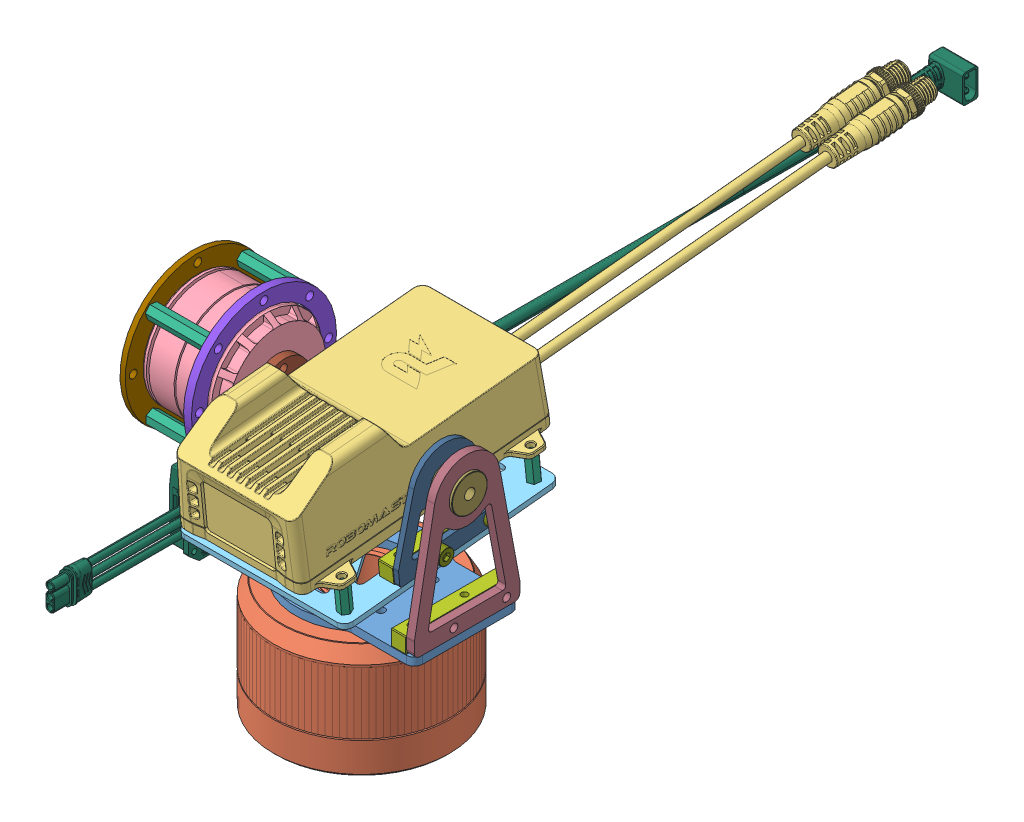
SolidWorks assembly 图传云台模块, configuration 默认. Lengths in mm.
Overall size (117.49 133.37 343.45).
28 component instances, 16 part files, 65 mates.
Components (placement in the parent):
- 6020电机传动板-1: 6020电机传动板 [默认] x (1 0 0) z (0 -1 0) size (80 50 3)
- RoboMaster GM6020 直流无刷电机-1: RoboMaster GM6020 直流无刷电机 [默认] at (0 72.0479 0) x (0.664685 0 -0.747124) z (0 1 0) size (66.7 66.7 45)
- RoboMaster 图传模块 VT02 2019-1: RoboMaster 图传模块 VT02 2019 [默认] at (0 34.0545 -1.0941) x (-1 0 0) z (0 0.099465 -0.995041) size (60 36.29 258.03)
- RoboMaster M3508直流无刷电机转子-1: RoboMaster M3508直流无刷电机转子 [默认] at (-11.659 32.3995 -13.3475) x (0 -0.790596 0.612338) z (-1 0 0) size (42 42 43.4)
- 图传安装板-1: 图传安装板 [默认] at (0 20.124 -2.4866) x (1 0 0) z (0 -0.995041 -0.099465) size (64 82 2)
- 304不锈钢柱-1: 304不锈钢柱 [M2*10] at (27 21.5184 33.8322) x (-0.601616 -0.079451 0.794824) z (0 -0.995041 -0.099465) size (4.62 4 10)
- 304不锈钢柱-2: 304不锈钢柱 [M2*10] at (-27 21.5184 33.8322) x (-0.601616 -0.079451 0.794824) z (0 -0.995041 -0.099465) size (4.62 4 10)
- 304不锈钢柱-3: 304不锈钢柱 [M2*10] at (27 28.6799 -37.8108) x (-0.956324 -0.029074 0.290859) z (0 -0.995041 -0.099465) size (4.62 4 10)
- 304不锈钢柱-4: 304不锈钢柱 [M2*10] at (-27 28.6799 -37.8108) x (0.570383 -0.081698 0.817306) z (0 -0.995041 -0.099465) size (4.62 4 10)
- 四孔直角转接件-1: 四孔直角转接件 [上交角件] at (-26 23.1091 -2.1882) x (1 0 0) z (0 -0.099465 0.995041) size (6 6 40)
- 四孔直角转接件-2: 四孔直角转接件 [上交角件] at (27 23.1091 -2.1882) x (1 0 0) z (0 -0.099465 0.995041) size (6 6 40)
- 云台转接板-1: 云台转接板 [默认] at (-37 45 0) x (0 0 1) z (-1 0 0) size (55 72.5 3.26)
- 3508定子安装板-1: 3508定子安装板 [默认] at (-64.1 45 0) x (0 0.707107 -0.707107) z (1 0 0) size (55 55 2)
- 云台旋转板-1: 云台旋转板 [默认] at (32 45 0) x (0 -0.099465 0.995041) z (-1 0 0) size (40 37.5 2)
- 3508传动板-1: 3508传动板 [默认] at (-32 45 0) x (0 0.099465 -0.995041) z (1 0 0) size (40 34.5 3)
- 法兰轴承-1: 法兰轴承 [4*12*4-1] at (41 45 0) x (0 0.036514 0.999333) z (0 -0.999333 0.036514) size (13.5 4 13.5)
- 转接板2-1: 转接板2 [默认] at (37 45 0) x (0 0 -1) z (1 0 0) size (40 57.5 3)
- 推力球轴承-1: 推力球轴承 [F4-9M 4*9*4] at (37 45 0) x (0 0.757396 -0.652956) z (0 0.652956 0.757396) size (9 4 9)
- 法兰轴承-2: 法兰轴承 [4*12*4-1] at (29 45 0) x (0 -0.234612 -0.972089) z (0 -0.972089 0.234612) size (13.5 4 13.5)
- 304不锈钢柱-5: 304不锈钢柱 [M3*22] at (-51 27.6759 17.3241) x (0 -0.514688 -0.857378) z (1 0 0) size (5.43 4.7 22)
- 304不锈钢柱-6: 304不锈钢柱 [M3*22] at (-51 27.6759 -17.3241) x (0 -0.372237 -0.928138) z (1 0 0) size (5.43 4.7 22)
- 304不锈钢柱-7: 304不锈钢柱 [M3*22] at (-51 62.3241 -17.3241) x (0 -0.251026 -0.96798) z (1 0 0) size (5.43 4.7 22)
- 304不锈钢柱-8: 304不锈钢柱 [M3*22] at (-51 62.3241 17.3241) x (0 -0.159705 -0.987165) z (1 0 0) size (5.43 4.7 22)
- 四孔直角转接件-3: 四孔直角转接件 [上交角件] at (34 3 0) size (6 6 40)
- 四孔直角转接件-4: 四孔直角转接件 [上交角件] at (-34 3 0) size (6 6 40)
- C620无刷电机调速器-1: C620无刷电机调速器 [默认] at (-45.4 6.2704 2.5313) x (0 0 1) z (0 1 0) size (343.45 13.81 26.13)
- 12.9级圆柱头螺钉-1: 12.9级圆柱头螺钉 [M3*8] at (35 22.6118 2.787) x (0 -0.455873 -0.890045) z (1 0 0) size (5.68 5.68 11)
- 12.9级圆柱头螺钉-2: 12.9级圆柱头螺钉 [M3*8] at (35 24.6011 -17.1138) x (0 -0.455873 -0.890045) z (1 0 0) size (5.68 5.68 11)
Mates (geometry in assembly coordinates):
- 重合1: coincident anti-aligned: plane of 6020电机传动板-1 through (0 -3 0) normal (0 -1 0); plane of RoboMaster GM6020 直流无刷电机-1 through (0 -3 0) normal (0 1 0)
- 同心1: concentric anti-aligned: cylinder of 6020电机传动板-1 through (0 -3 0) axis (0 1 0) radius 15; cylinder of RoboMaster GM6020 直流无刷电机-1 through (0 -0.95 0) axis (0 -1 0) radius 9
- 对称1: symmetric aligned: plane of RoboMaster 图传模块 VT02 2019-1 through (24 38.8289 -48.8561) normal (1 0 0); plane of RoboMaster 图传模块 VT02 2019-1 through (-24 29.2802 46.6679) normal (-1 0 0)
- 距离1: distance = 10 mm anti-aligned: plane of 图传安装板-1 through (0 20.124 -2.4866) normal (0 0.995041 0.099465); plane of RoboMaster 图传模块 VT02 2019-1 through (0 30.0744 -1.492) normal (0 -0.995041 -0.099465)
- 同心3: concentric aligned: cylinder of RoboMaster 图传模块 VT02 2019-1 through (27 26.4936 34.3295) axis (0 0.995041 0.099465) radius 1.35; cylinder of 图传安装板-1 through (27 14.5532 33.1359) axis (0 0.995041 0.099465) radius 1.25
- 同心4: concentric anti-aligned: cylinder of RoboMaster 图传模块 VT02 2019-1 through (-27 26.4936 34.3295) axis (0 -0.995041 -0.099465) radius 1.35; cylinder of 图传安装板-1 through (-27 14.5532 33.1359) axis (0 0.995041 0.099465) radius 1.25
- 重合3: coincident anti-aligned: plane of 图传安装板-1 through (0 20.124 -2.4866) normal (0 0.995041 0.099465); plane of 304不锈钢柱-1 through (27 16.5432 33.3349) normal (0 -0.995041 -0.099465)
- 同心5: concentric anti-aligned: cylinder of 图传安装板-1 through (27 14.5532 33.1359) axis (0 0.995041 0.099465) radius 1.25; cylinder of 304不锈钢柱-1 through (27 16.5432 33.3349) axis (0 -0.995041 -0.099465) radius 0.8
- 重合4: coincident anti-aligned: plane of 图传安装板-1 through (0 20.124 -2.4866) normal (0 0.995041 0.099465); plane of 304不锈钢柱-2 through (-27 16.5432 33.3349) normal (0 -0.995041 -0.099465)
- 同心6: concentric anti-aligned: cylinder of 图传安装板-1 through (-27 14.5532 33.1359) axis (0 0.995041 0.099465) radius 1.25; cylinder of 304不锈钢柱-2 through (-27 16.5432 33.3349) axis (0 -0.995041 -0.099465) radius 0.8
- 同心7: concentric aligned: cylinder of RoboMaster 图传模块 VT02 2019-1 through (27 33.6551 -37.3135) axis (0 -0.995041 -0.099465) radius 1.35; cylinder of 304不锈钢柱-3 through (27 23.7047 -38.3081) axis (0 -0.995041 -0.099465) radius 0.8
- 重合5: coincident anti-aligned: plane of 图传安装板-1 through (0 20.124 -2.4866) normal (0 0.995041 0.099465); plane of 304不锈钢柱-3 through (27 23.7047 -38.3081) normal (0 -0.995041 -0.099465)
- 同心8: concentric anti-aligned: cylinder of 图传安装板-1 through (-27 21.7146 -38.507) axis (0 0.995041 0.099465) radius 1.25; cylinder of 304不锈钢柱-4 through (-27 23.7047 -38.3081) axis (0 -0.995041 -0.099465) radius 0.8
- 重合6: coincident anti-aligned: plane of 图传安装板-1 through (0 20.124 -2.4866) normal (0 0.995041 0.099465); plane of 304不锈钢柱-4 through (-27 23.7047 -38.3081) normal (0 -0.995041 -0.099465)
- 重合7: coincident anti-aligned: plane of 图传安装板-1 through (0 20.124 -2.4866) normal (0 0.995041 0.099465); plane of 四孔直角转接件-1 through (-29 18.1347 17.4142) normal (0 -0.995041 -0.099465)
- 宽度1: width aligned: plane of 图传安装板-1 through (-32 14.0558 38.1111) normal (0 -0.099465 0.995041); plane of 四孔直角转接件-1 through (-32 22.212 -43.4822) normal (0 0.099465 -0.995041); plane of 图传安装板-1 through (-26 21.1198 17.7126) normal (0 -0.099465 0.995041); plane of 四孔直角转接件-1 through (-26 25.0984 -22.0891) normal (0 0.099465 -0.995041)
- 重合8: coincident anti-aligned: plane of 图传安装板-1 through (0 20.124 -2.4866) normal (0 0.995041 0.099465); plane of 四孔直角转接件-2 through (24 18.1347 17.4142) normal (0 -0.995041 -0.099465)
- 重合9: coincident aligned: plane of 四孔直角转接件-1 through (-26 21.1198 17.7126) normal (0 -0.099465 0.995041); plane of 四孔直角转接件-2 through (27 21.1198 17.7126) normal (0 -0.099465 0.995041)
- 重合10: coincident aligned: plane of 6020电机传动板-1 through (-40 47.1699 -20) normal (-1 0 0); plane of 云台转接板-1 through (-40 45 0) normal (-1 0 0)
- 重合11: coincident anti-aligned: plane of 6020电机传动板-1 through (0 0 0) normal (0 1 0); plane of 云台转接板-1 through (-40 0 -20) normal (0 -1 0)
- 对称2: symmetric aligned: plane of 6020电机传动板-1 through (-40 47.1699 20) normal (0 0 1); plane of 云台转接板-1 through (-40 47.1699 -20) normal (0 0 -1); plane of 6020电机传动板-1 through (-37 45 0) normal (0 0 1)
- 同心9: concentric aligned: cylinder of RoboMaster M3508直流无刷电机转子-1 through (-60.1 45 0) axis (-1 0 0) radius 21; cylinder of 云台转接板-1 through (-37 45 0) axis (-1 0 0) radius 21.5
- 同心10: concentric anti-aligned: cylinder of RoboMaster M3508直流无刷电机转子-1 through (-64.1 45 0) axis (1 0 0) radius 13.4; cylinder of 3508定子安装板-1 through (-62.1 45 0) axis (-1 0 0) radius 13.5
- 重合12: coincident anti-aligned: plane of RoboMaster M3508直流无刷电机转子-1 through (-62.1 45 0) normal (-1 0 0); plane of 3508定子安装板-1 through (-62.1 45 0) normal (1 0 0)
- 重合13: coincident anti-aligned: plane of 四孔直角转接件-2 through (30 18.1347 17.4142) normal (1 0 0); plane of 云台旋转板-1 through (30 45 0) normal (-1 0 0)
- 重合14: coincident anti-aligned: plane of 图传安装板-1 through (0 20.124 -2.4866) normal (0 0.995041 0.099465); plane of 云台旋转板-1 through (30 22.1133 -22.3874) normal (0 -0.995041 -0.099465)
- 重合15: coincident aligned: plane of 四孔直角转接件-2 through (27 21.1198 17.7126) normal (0 -0.099465 0.995041); plane of 云台旋转板-1 through (30 18.1347 17.4142) normal (0 -0.099465 0.995041)
- 同心11: concentric anti-aligned: cylinder of RoboMaster M3508直流无刷电机转子-1 through (-60.1 45 0) axis (-1 0 0) radius 21; cylinder of 云台旋转板-1 through (30 45 0) axis (1 0 0) radius 6
- 重合16: coincident aligned: plane of 图传安装板-1 through (32 22.212 -43.4822) normal (1 0 0); plane of 云台旋转板-1 through (32 45 0) normal (1 0 0)
- 重合17: coincident anti-aligned: plane of 四孔直角转接件-1 through (-29 18.1347 17.4142) normal (-1 0 0); plane of 3508传动板-1 through (-29 45 0) normal (1 0 0)
- 重合18: coincident aligned: plane of 四孔直角转接件-1 through (-26 21.1198 17.7126) normal (0 -0.099465 0.995041); plane of 3508传动板-1 through (-29 18.1347 17.4142) normal (0 -0.099465 0.995041)
- 重合19: coincident aligned: plane of 图传安装板-1 through (-32 22.212 -43.4822) normal (-1 0 0); plane of 3508传动板-1 through (-32 45 0) normal (-1 0 0)
- 重合20: coincident anti-aligned: plane of 图传安装板-1 through (0 20.124 -2.4866) normal (0 0.995041 0.099465); plane of 3508传动板-1 through (-29 18.1347 17.4142) normal (0 -0.995041 -0.099465)
- 重合21: coincident anti-aligned: plane of RoboMaster M3508直流无刷电机转子-1 through (-32 45 0) normal (1 0 0); plane of 3508传动板-1 through (-32 45 0) normal (-1 0 0)
- 重合22: coincident aligned: plane of 6020电机传动板-1 through (40 47.1699 -20) normal (1 0 0); plane of 转接板2-1 through (40 45 0) normal (1 0 0)
- 重合23: coincident anti-aligned: plane of 6020电机传动板-1 through (0 0 0) normal (0 1 0); plane of 转接板2-1 through (40 0 20) normal (0 -1 0)
- 重合24: coincident aligned: plane of 6020电机传动板-1 through (15 47.1699 20) normal (0 0 1); plane of 转接板2-1 through (40 0 20) normal (0 0 1)
- 同心12: concentric anti-aligned: cylinder of 法兰轴承-1 through (37 45 0) axis (1 0 0) radius 6; cylinder of 转接板2-1 through (40 45 0) axis (-1 0 0) radius 6
- 重合25: coincident anti-aligned: plane of 法兰轴承-1 through (40 45 0) normal (-1 0 0); plane of 转接板2-1 through (40 45 0) normal (1 0 0)
- 同心13: concentric anti-aligned: cylinder of 云台旋转板-1 through (30 45 0) axis (1 0 0) radius 6; cylinder of 法兰轴承-2 through (33 45 0) axis (-1 0 0) radius 6
- 重合26: coincident anti-aligned: plane of 云台旋转板-1 through (30 45 0) normal (-1 0 0); plane of 法兰轴承-2 through (30 45 0) normal (1 0 0)
- 同心14: concentric aligned: cylinder of 法兰轴承-1 through (37 45 0) axis (1 0 0) radius 2; cylinder of 推力球轴承-1 through (33 45 0) axis (1 0 0) radius 2
- 宽度2: width anti-aligned: plane of 推力球轴承-1 through (33 45 0) normal (-1 0 0); plane of 法兰轴承-2 through (37 45 0) normal (1 0 0); plane of 推力球轴承-1 through (33 45 0) normal (1 0 0); plane of 转接板2-1 through (37 45 0) normal (-1 0 0)
- 同心15: concentric anti-aligned: cylinder of 云台转接板-1 through (-37 45 24.5) axis (-1 0 0) radius 1.525; cylinder of 3508定子安装板-1 through (-64.1 45 24.5) axis (1 0 0) radius 1.525
- 同心16: concentric anti-aligned: cylinder of 3508定子安装板-1 through (-64.1 27.6759 17.3241) axis (1 0 0) radius 1.525; cylinder of 304不锈钢柱-5 through (-62 27.6759 17.3241) axis (-1 0 0) radius 1.25
- 重合27: coincident anti-aligned: plane of 云台转接板-1 through (-40 45 0) normal (-1 0 0); plane of 304不锈钢柱-5 through (-40 27.6759 17.3241) normal (1 0 0)
- 重合28: coincident anti-aligned: plane of 云台转接板-1 through (-40 45 0) normal (-1 0 0); plane of 304不锈钢柱-6 through (-40 27.6759 -17.3241) normal (1 0 0)
- 同心18: concentric anti-aligned: cylinder of 3508定子安装板-1 through (-64.1 27.6759 -17.3241) axis (1 0 0) radius 1.525; cylinder of 304不锈钢柱-6 through (-62 27.6759 -17.3241) axis (-1 0 0) radius 1.25
- 重合29: coincident anti-aligned: plane of 云台转接板-1 through (-40 45 0) normal (-1 0 0); plane of 304不锈钢柱-7 through (-40 62.3241 -17.3241) normal (1 0 0)
- 同心19: concentric anti-aligned: cylinder of 3508定子安装板-1 through (-64.1 62.3241 -17.3241) axis (1 0 0) radius 1.525; cylinder of 304不锈钢柱-7 through (-62 62.3241 -17.3241) axis (-1 0 0) radius 1.25
- 重合30: coincident anti-aligned: plane of 云台转接板-1 through (-40 45 0) normal (-1 0 0); plane of 304不锈钢柱-8 through (-40 62.3241 17.3241) normal (1 0 0)
- 同心20: concentric anti-aligned: cylinder of 3508定子安装板-1 through (-64.1 62.3241 17.3241) axis (1 0 0) radius 1.525; cylinder of 304不锈钢柱-8 through (-62 62.3241 17.3241) axis (-1 0 0) radius 1.25
- 同心21: concentric anti-aligned: cylinder of RoboMaster M3508直流无刷电机转子-1 through (-62.1 28.0963 4.5293) axis (-1 0 0) radius 1.5; cylinder of 3508定子安装板-1 through (-64.1 28.0963 4.5293) axis (1 0 0) radius 1.525
- 重合32: coincident anti-aligned: plane of 6020电机传动板-1 through (0 0 0) normal (0 1 0); plane of 四孔直角转接件-3 through (31 0 20) normal (0 -1 0)
- 重合33: coincident aligned: plane of 6020电机传动板-1 through (15 47.1699 20) normal (0 0 1); plane of 四孔直角转接件-3 through (34 3 20) normal (0 0 1)
- 重合34: coincident anti-aligned: plane of 转接板2-1 through (37 45 0) normal (-1 0 0); plane of 四孔直角转接件-3 through (37 0 20) normal (1 0 0)
- 重合35: coincident aligned: plane of 6020电机传动板-1 through (-40 47.1699 20) normal (0 0 1); plane of 四孔直角转接件-4 through (-34 3 20) normal (0 0 1)
- 重合36: coincident anti-aligned: plane of 云台转接板-1 through (-37 45 0) normal (1 0 0); plane of 四孔直角转接件-4 through (-37 0 20) normal (-1 0 0)
- 重合37: coincident anti-aligned: plane of 6020电机传动板-1 through (0 0 0) normal (0 1 0); plane of 四孔直角转接件-4 through (-37 0 20) normal (0 -1 0)
- 重合38: coincident anti-aligned: plane of 云台转接板-1 through (-40 45 0) normal (-1 0 0); plane of C620无刷电机调速器-1 through (-40 6.2704 0.8313) normal (1 0 0)
- 平行2: parallel anti-aligned: plane of 6020电机传动板-1 through (0 0 0) normal (0 1 0); plane of C620无刷电机调速器-1 through (-41 -6.6296 -19.6687) normal (0 -1 0)
- 同心22: concentric anti-aligned: cylinder of 云台旋转板-1 through (22 22.6118 2.787) axis (1 0 0) radius 1.515; cylinder of 12.9级圆柱头螺钉-1 through (24 22.6118 2.787) axis (-1 0 0) radius 1.5
- 重合39: coincident anti-aligned: plane of 云台旋转板-1 through (32 45 0) normal (1 0 0); plane of 12.9级圆柱头螺钉-1 through (32 25.1395 1.4923) normal (-1 0 0)
- 同心231: concentric anti-aligned: cylinder of 云台旋转板-1 through (22 24.6011 -17.1138) axis (1 0 0) radius 1.515; cylinder of 12.9级圆柱头螺钉-2 through (24 24.6011 -17.1138) axis (-1 0 0) radius 2.84
- 重合401: coincident anti-aligned: plane of 云台旋转板-1 through (32 45 0) normal (1 0 0); plane of 12.9级圆柱头螺钉-2 through (32 27.1288 -18.4085) normal (-1 0 0)
